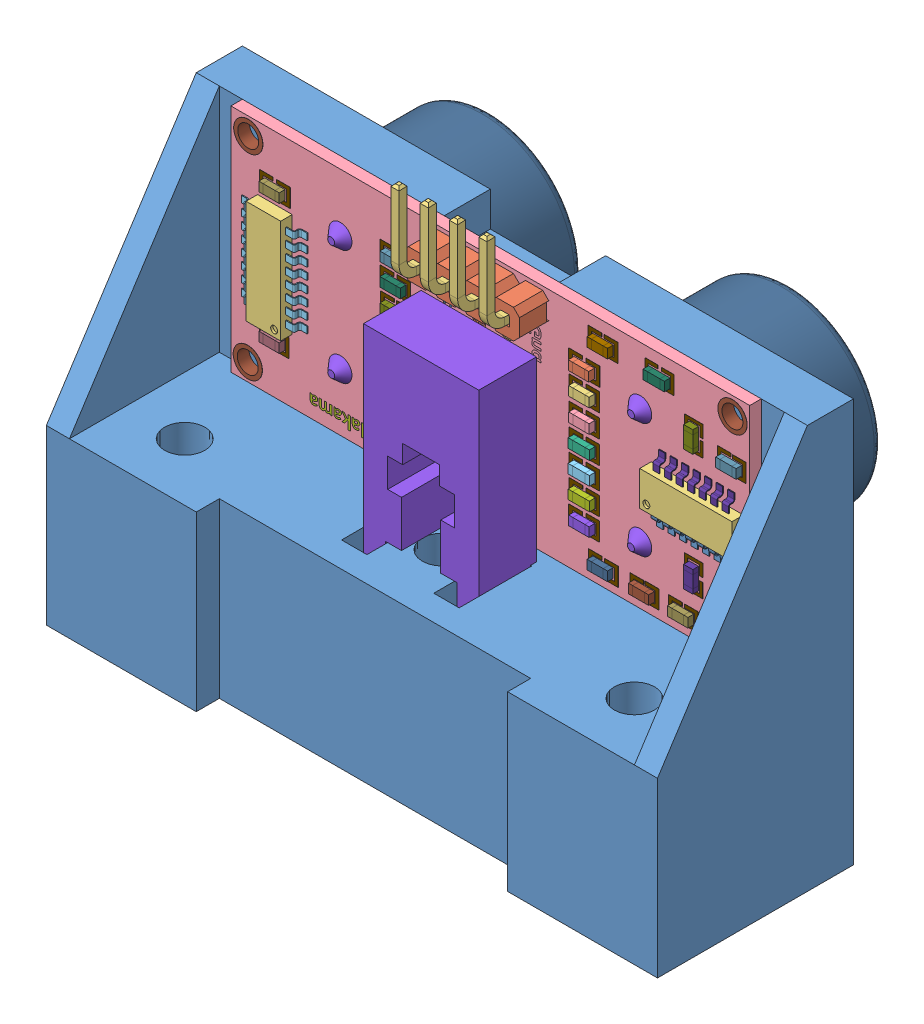
SolidWorks assembly cummat_giua, configuration Default. Lengths in mm.
Overall size (53 40.57 25).
64 component instances, 62 part files, 6 mates.
Components (placement in the parent):
- ga lap ultrasonic v5-1: ga lap ultrasonic v5 [Default] at (-41.4429 24.5912 58.324) size (53 35 17)
- HC-04HC-04-1: HC-04HC-04 [Default] at (-27.3624 33.2981 63.324) x (1 0 0) z (0 0 -1) size (45 25.57 17.46)
  - HC-04HC-04.stp-1: HC-04HC-04.stp [Default] at origin size (45 25.57 17.46)
    - HC-04Array.stp-1: HC-04Array.stp [Default] at origin size (10.16 2.54 2.54)
    - HC-04Array001.stp-1: HC-04Array001.stp [Default] at (0 0 1) size (8.32 7.52 6.46)
    - HC-04Placa.stp-1: HC-04Placa.stp [Default] at origin size (45 20 1)
    - HC-04Pad003.stp-1: HC-04Pad003.stp [Default] at (0 0 1) size (10.52 3.38 0.2)
    - HC-04Fillet.stp-1: HC-04Fillet.stp [Default] at (0 0 1) size (10.1 2.84 3)
    - HC-04Array002.stp-1: HC-04Array002.stp [Default] at origin size (9.62 2 1)
    - HC-04Array003.stp-1: HC-04Array003.stp [Default] at (0 0 1) size (28 12 0.8)
    - HC-04Fusion.stp-1: HC-04Fusion.stp [Default] at origin size (6 2 1)
    - HC-04Fillet001.stp-1: HC-04Fillet001.stp [Default] at (0 0 1) size (42 16 12)
    - HC-04Pad005.stp-1: HC-04Pad005.stp [Default] at (0 0 1) size (39.16 13 0.2)
    - HC-04Pad006.stp-1: HC-04Pad006.stp [Default] at (0 0 1) size (35.01 9.04 7)
    - HC-04Fusion001.stp-1: HC-04Fusion001.stp [Default] at (0 0 8) size (31 5 1.5)
    - HC-04Clone_of_Fusion002.stp-1: HC-04Clone_of_Fusion002.stp [Default] at (47.2 -5.5 12.6) size (13 13 0.15)
    - HC-04Clone_of_Fusion003.stp-1: HC-04Clone_of_Fusion003.stp [Default] at (21.2 -5.5 12.6) size (13 13 0.15)
    - HC-04Array005.stp-1: HC-04Array005.stp [Default] at origin size (9.62 2 1)
    - HC-04Array002002.stp-1: HC-04Array002002.stp [Default] at (-5.9 0.1 0.15) size (6.57 1.4 0.56)
    - HC-04Clone_of_Array002002.stp-1: HC-04Clone_of_Array002002.stp [Default] at (-23.9 0.1 0.15) size (6.57 1.4 0.56)
    - HC-04Array002003.stp-1: HC-04Array002003.stp [Default] at (-6.05 0 0.15) size (6.57 1.4 0.56)
    - HC-04Clone_of_Array002003.stp-1: HC-04Clone_of_Array002003.stp [Default] at (-24.05 0 0.15) size (6.57 1.4 0.56)
    - HC-04Integrados.stp-1: HC-04Integrados.stp [Default] at origin size (42.14 9 1)
    - HC-04ShapeString.stp-1: HC-04ShapeString.stp [Default] at (-3.2 -7 1.01) x (0 1 0) z (0 0 1) size (2.53 1.13 0.01)
    - HC-04ShapeString001.stp-1: HC-04ShapeString001.stp [Default] at (-0.6 -7 1.01) x (0 1 0) z (0 0 1) size (2.66 1.45 0.01)
    - HC-04ShapeString002.stp-1: HC-04ShapeString002.stp [Default] at (1.9 -7 1.01) x (0 1 0) z (0 0 1) size (3.21 1.16 0.01)
    - HC-04ShapeString003.stp-1: HC-04ShapeString003.stp [Default] at (4.5 -7 1.01) x (0 1 0) z (0 0 1) size (2.71 1.16 0.01)
    - HC-04ShapeString004.stp-1: HC-04ShapeString004.stp [Default] at (-19.5 -9.3 1.01) size (1.84 2.34 0.01)
    - HC-04ShapeString005.stp-1: HC-04ShapeString005.stp [Default] at (17.5 -9.3 1.01) size (1.82 2.34 0.01)
    - HC-04ShapeString006.stp-1: HC-04ShapeString006.stp [Default] at (-3 3.7 1.01) size (5.52 1.41 0.01)
    - HC-04Pad008.stp-1: HC-04Pad008.stp [Default] at (0 0 -0.01) size (44.56 19.6 1.02)
    - HC-04Scale004.stp-1: HC-04Scale004.stp [Default] at (-1.9 -21.5 -1.5) x (0 1 0) z (0 0 1) size (0.8 1.77 0.5)
    - HC-04Scale027.stp-1: HC-04Scale027.stp [Default] at (-1.9 -10.2323 -1.5) x (0 1 0) z (0 0 1) size (0.8 1.77 0.5)
    - HC-04Scale028.stp-1: HC-04Scale028.stp [Default] at (8.5984 -21.5 -1.5) x (0 1 0) z (0 0 1) size (0.8 1.77 0.5)
    - HC-04Scale029.stp-1: HC-04Scale029.stp [Default] at (8.5984 -19.5867 -1.5) x (0 1 0) z (0 0 1) size (0.8 1.77 0.5)
    - HC-04Scale030.stp-1: HC-04Scale030.stp [Default] at (8.5984 -17.5982 -1.5) x (0 1 0) z (0 0 1) size (0.8 1.77 0.5)
    - HC-04Scale031.stp-1: HC-04Scale031.stp [Default] at (8.5984 -15.6427 -1.5) x (0 1 0) z (0 0 1) size (0.8 1.77 0.5)
    - HC-04Scale032.stp-1: HC-04Scale032.stp [Default] at (8.5984 -11.6848 -1.5) x (0 1 0) z (0 0 1) size (0.8 1.77 0.5)
    - HC-04Scale033.stp-1: HC-04Scale033.stp [Default] at (-26.74 -2 -1.5) x (0 1 0) z (0 0 1) size (0.8 1.85 0.5)
    - HC-04Scale034.stp-1: HC-04Scale034.stp [Default] at (24.9371 -21.5 -1.5) x (0 1 0) z (0 0 1) size (0.8 1.77 0.5)
    - HC-04Scale035.stp-1: HC-04Scale035.stp [Default] at (24.9691 -19.5867 -1.5) x (0 1 0) z (0 0 1) size (0.8 1.77 0.5)
    - HC-04Scale036.stp-1: HC-04Scale036.stp [Default] at (24.9742 -17.5982 -1.5) x (0 1 0) z (0 0 1) size (0.8 1.77 0.5)
    - HC-04Scale037.stp-1: HC-04Scale037.stp [Default] at (-10.4013 -2 -1.5) x (0 1 0) z (0 0 1) size (0.8 1.85 0.5)
    - HC-04Scale038.stp-1: HC-04Scale038.stp [Default] at (-10.4013 -3.9266 -1.5) x (0 1 0) z (0 0 1) size (0.8 1.85 0.5)
    - HC-04Scale039.stp-1: HC-04Scale039.stp [Default] at (-10.4013 -0.0734 -1.5) x (0 1 0) z (0 0 1) size (0.8 1.85 0.5)
    - HC-04Scale040.stp-1: HC-04Scale040.stp [Default] at (24.9742 -9.855 -1.5) x (0 1 0) z (0 0 1) size (0.8 1.77 0.5)
    - HC-04Scale041.stp-1: HC-04Scale041.stp [Default] at (26.5673 -24.0564 -1.5) x (0 1 0) z (0 0 1) size (0.8 1.77 0.5)
    - HC-04Scale042.stp-1: HC-04Scale042.stp [Default] at (26.5673 -7.3333 -1.5) x (0 1 0) z (0 0 1) size (0.8 1.77 0.5)
    - HC-04Scale043.stp-1: HC-04Scale043.stp [Default] at (30.1435 -7.3333 -1.5) x (0 1 0) z (0 0 1) size (0.8 1.77 0.5)
    - HC-04Scale044.stp-1: HC-04Scale044.stp [Default] at (33.5459 -7.3333 -1.5) x (0 1 0) z (0 0 1) size (0.8 1.77 0.5)
    - HC-04Scale045.stp-1: HC-04Scale045.stp [Default] at (37.7181 -11.1827 -1.5) x (0 1 0) z (0 0 1) size (0.8 1.77 0.5)
    - HC-04Scale046.stp-1: HC-04Scale046.stp [Default] at (37.7181 -20.5932 -1.5) x (0 1 0) z (0 0 1) size (0.8 1.77 0.5)
    - HC-04Scale047.stp-1: HC-04Scale047.stp [Default] at (-3.9042 -12.3288 -1.5) x (0 1 0) z (0 0 1) size (0.8 1.85 0.5)
    - HC-04Scale048.stp-1: HC-04Scale048.stp [Default] at (13.5402 13.2894 -1.5) size (0.8 1.85 0.5)
    - HC-04Scale049.stp-1: HC-04Scale049.stp [Default] at (13.5402 23.7909 -1.5) size (0.8 1.85 0.5)
    - HC-04Pad009.stp-1: HC-04Pad009.stp [Default] x (1 0 0) z (0 0 -1) size (42.21 18.43 0.01)
    - HC-04ShapeString007.stp-1: HC-04ShapeString007.stp [Default] at (-3.2 -7 -0.1) x (0 1 0) z (0 0 1) size (2.53 1.13 0.01)
    - HC-04ShapeString008.stp-1: HC-04ShapeString008.stp [Default] at (-0.6 -7 -0.1) x (0 1 0) z (0 0 1) size (2.66 1.45 0.01)
    - HC-04ShapeString009.stp-1: HC-04ShapeString009.stp [Default] at (1.9 -7 -0.1) x (0 1 0) z (0 0 1) size (3.21 1.16 0.01)
    - HC-04ShapeString010.stp-1: HC-04ShapeString010.stp [Default] at (4.5 -7 -0.1) x (0 1 0) z (0 0 1) size (2.71 1.16 0.01)
    - HC-04Fusion002.stp-1: HC-04Fusion002.stp [Default] at origin size (5.7 7.57 0.56)
    - HC-04ShapeString011.stp-1: HC-04ShapeString011.stp [Default] at (-17.5 8.4 1.1) size (7.91 1.16 0.01)
    - HC-04ShapeString012.stp-1: HC-04ShapeString012.stp [Default] at (-7.5 8 -0.1) x (-1 0 0) z (0 0 -1) size (7.91 1.16 0.01)
- 12.ganh-1: 12.ganh [Default] at (-27.3624 29.1981 64.324) x (1 0 0) z (0 -1 0) size (10 5 19)
Mates (geometry in assembly coordinates):
- Coincident1: coincident anti-aligned: plane of ga lap ultrasonic v5-1 through (-41.4429 24.5912 62.324) normal (0 0 1); plane of HC-04HC-04-1/HC-04HC-04.stp-1/HC-04Placa.stp-1 through (-49.8624 23.2981 62.324) normal (0 0 -1)
- Width1: width anti-aligned: plane of HC-04HC-04-1/HC-04HC-04.stp-1/HC-04Placa.stp-1 through (-49.8624 43.2981 63.324) normal (-1 0 0); plane of HC-04HC-04-1/HC-04HC-04.stp-1/HC-04Placa.stp-1 through (-4.8624 23.2981 63.324) normal (1 0 0); plane of ga lap ultrasonic v5-1 through (-0.8624 43.2981 75.324) normal (1 0 0); plane of ga lap ultrasonic v5-1 through (-53.8624 43.2981 75.324) normal (-1 0 0)
- Coincident2: coincident anti-aligned: plane of ga lap ultrasonic v5-1 through (-27.3624 23.2981 75.324) normal (0 1 0); plane of HC-04HC-04-1/HC-04HC-04.stp-1/HC-04Placa.stp-1 through (-49.8624 23.2981 63.324) normal (0 -1 0)
- Coincident3: coincident anti-aligned: plane of ga lap ultrasonic v5-1 through (-27.3624 23.2981 75.324) normal (0 1 0); plane of 12.ganh-1 through (-27.3624 23.2981 69.324) normal (0 -1 0)
- Coincident4: coincident anti-aligned: plane of HC-04HC-04-1/HC-04HC-04.stp-1/HC-04Integrados.stp-1 through (-31.3624 31.7981 64.324) normal (0 0 1); plane of 12.ganh-1 through (-27.3624 29.1981 64.324) normal (0 0 -1)
- Width2: width aligned: plane of ga lap ultrasonic v5-1 through (-53.8624 43.2981 75.324) normal (-1 0 0); plane of ga lap ultrasonic v5-1 through (-0.8624 43.2981 75.324) normal (1 0 0); plane of 12.ganh-1 through (-32.3624 29.1981 69.324) normal (-1 0 0); plane of 12.ganh-1 through (-22.3624 29.1981 69.324) normal (1 0 0)
